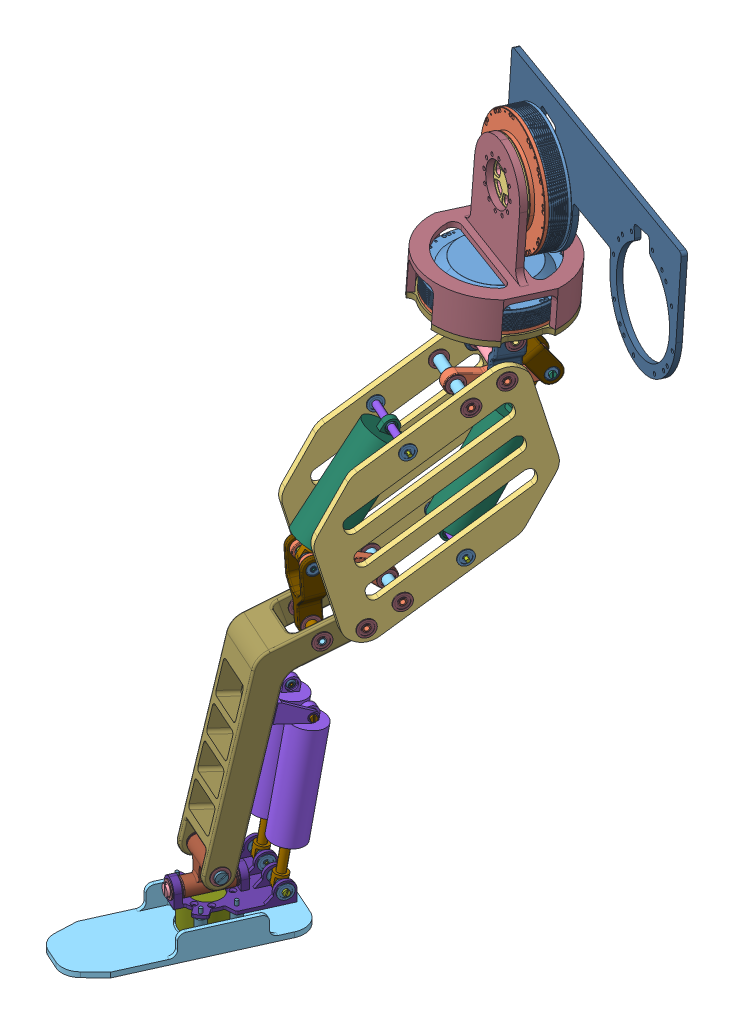
SolidWorks assembly 腿部总装, configuration 默认. Lengths in mm. (continued)
Mates (geometry in assembly coordinates): (continued)
- 同心60: concentric anti-aligned: cylinder of 轴承_NSK635-11 through (543.2359 479.3983 -8003.7197) axis (-0.911939 0 -0.410325) radius 2.5; cylinder of 膝关节5mm轴套2-3 through (539.2336 479.3983 -8005.5205) axis (0.911939 0 0.410325) radius 5
- 重合124: coincident anti-aligned: plane of 轴承_NSK635-14 through (539.0094 476.9588 -8005.0222) normal (0.911939 0 0.410325); plane of 膝关节5mm轴套2-3 through (539.2336 479.3983 -8005.5205) normal (-0.911939 0 -0.410325)
- 同心61: concentric aligned: circle of 膝髋推杆-1/脚踝推杆球头-2; cylinder of 膝关节5mm轴套3-2 through (526.0105 479.3983 -8011.4702) axis (0.911939 0 0.410325) radius 5
- 重合125: coincident anti-aligned: plane of 膝髋推杆-1/脚踝推杆球头-2 through (526.0105 479.3983 -8011.4702) normal (0.911939 0 0.410325); plane of 膝关节5mm轴套3-2 through (526.0105 479.3983 -8011.4702) normal (-0.911939 0 -0.410325)
- 同心62: concentric aligned: cylinder of 大腿侧板-1 through (511.6182 660.5079 -8116.57) axis (-0.911939 0 -0.410325) radius 9.5; cylinder of 轴承_NSK635-16 through (509.3577 659.5509 -8117.9101) axis (-0.911939 0 -0.410325) radius 9.5
- 重合126: coincident aligned: plane of 大腿侧板-1 through (425.784 514.1163 -7935.5535) normal (-0.911939 0 -0.410325); plane of 轴承_NSK635-16 through (507.193 650.3066 -8116.4834) normal (-0.911939 0 -0.410325)
- 同心63: concentric anti-aligned: cylinder of 大腿侧板-1 through (511.6182 660.5079 -8116.57) axis (0.911939 0 0.410325) radius 9.5; cylinder of 轴承_NSK635-15 through (513.0055 659.5509 -8116.2688) axis (-0.911939 0 -0.410325) radius 9.5
- 重合127: coincident aligned: plane of 大腿侧板-1 through (434.9033 514.1163 -7931.4502) normal (0.911939 0 0.410325); plane of 轴承_NSK635-15 through (516.5522 651.7135 -8112.9131) normal (0.911939 0 0.410325)
- 同心64: concentric anti-aligned: cylinder of 轴承_NSK635-15 through (513.0055 659.5509 -8116.2688) axis (-0.911939 0 -0.410325) radius 2.5; cylinder of 膝关节5mm轴套4-1 through (518.4578 660.5079 -8113.4926) axis (0.911939 0 0.410325) radius 5
- 重合128: coincident anti-aligned: plane of 膝髋推杆-1/脚踝推杆球头-1 through (559.5325 633.0528 -8107.9058) normal (-0.911939 0 -0.410325); plane of 膝关节5mm轴套4-1 through (559.5325 633.0528 -8107.9058) normal (0.911939 0 0.410325)
- 同心65: concentric anti-aligned: cylinder of 大腿侧板-1 through (543.7977 674.861 -8197.8367) axis (0.911939 0 0.410325) radius 11; cylinder of 膝关节U型架后侧-2 through (629.6228 674.861 -8159.2199) axis (-0.911939 0 -0.410325) radius 11
- 重合129: coincident aligned: plane of 膝关节U型架后侧-1 through (553.0875 467.2754 -8064.9462) normal (0.911939 0 0.410325); plane of 膝关节U型架后侧-2 through (621.3197 658.4644 -8216.5909) normal (0.911939 0 0.410325)
- 同心66: concentric aligned: cylinder of 膝髋推杆-2/脚踝推杆球头-2 through (633.731 675.7893 -8275.2477) axis (0.911939 0 0.410325) radius 2.5; cylinder of 膝关节U型架后侧-2 through (650.6019 675.7893 -8267.6567) axis (0.911939 0 0.410325) radius 9.5
- 同心67: concentric anti-aligned: cylinder of 膝关节U型架后侧-2 through (650.6019 675.7893 -8267.6567) axis (0.911939 0 0.410325) radius 9.5; cylinder of 轴承_NSK635-19 through (651.8683 675.7893 -8267.0868) axis (-0.911939 0 -0.410325) radius 9.5
- 重合130: coincident aligned: plane of 膝关节U型架后侧-2 through (656.536 664.3447 -8266.2225) normal (0.911939 0 0.410325); plane of 轴承_NSK635-19 through (655.356 667.9828 -8263.6001) normal (0.911939 0 0.410325)
- 同心68: concentric aligned: cylinder of 膝关节U型架后侧-2 through (626.8915 675.7893 -8278.3251) axis (-0.911939 0 -0.410325) radius 9.5; cylinder of 轴承_NSK635-20 through (622.6862 675.7893 -8280.2172) axis (-0.911939 0 -0.410325) radius 9.5
- 重合131: coincident aligned: plane of 膝关节U型架后侧-2 through (602.1794 659.6159 -8238.0256) normal (-0.911939 0 -0.410325); plane of 轴承_NSK635-20 through (620.5678 666.519 -8278.8934) normal (-0.911939 0 -0.410325)
- 距离5: distance = 6.5 mm anti-aligned: plane of 膝髋推杆-2/脚踝推杆球头-2 through (634.6429 675.7893 -8274.8373) normal (-0.911939 0 -0.410325); plane of 膝关节U型架后侧-2 through (629.1778 664.3447 -8278.5323) normal (0.911939 0 0.410325)
- 重合133: coincident aligned: circle of 膝关节U型架后侧-2; circle of 轴承_NSK6900NR-27
- 重合134: coincident aligned: circle of 膝关节U型架后侧-2; circle of 轴承_NSK6900NR-26
- 同心69: concentric aligned: cylinder of 大腿侧板-1 through (544.8687 471.6931 -8190.4684) axis (0.911939 0 0.410325) radius 9.5; cylinder of 膝髋推杆-2/脚踝推杆球头-1 through (587.0459 471.6931 -8171.4909) axis (0.911939 0 0.410325) radius 2.5
- 同心70: concentric anti-aligned: cylinder of 大腿侧板-1 through (524.9446 487.9356 -8146.1876) axis (0.911939 0 0.410325) radius 9.5; cylinder of 轴承_NSK635-22 through (526.8516 487.2218 -8147.0414) axis (-0.911939 0 -0.410325) radius 9.5
- 重合135: coincident aligned: plane of 大腿侧板-1 through (434.9033 514.1163 -7931.4502) normal (0.911939 0 0.410325); plane of 轴承_NSK635-22 through (530.5858 479.3045 -8144.1025) normal (0.911939 0 0.410325)
- 同心71: concentric aligned: cylinder of 大腿侧板-1 through (524.9446 487.9356 -8146.1876) axis (-0.911939 0 -0.410325) radius 9.5; cylinder of 轴承_NSK635-23 through (523.2038 487.2218 -8148.6827) axis (-0.911939 0 -0.410325) radius 9.5
- 重合136: coincident aligned: plane of 大腿侧板-1 through (425.784 514.1163 -7935.5535) normal (-0.911939 0 -0.410325); plane of 轴承_NSK635-23 through (521.3781 477.82 -8148.0095) normal (-0.911939 0 -0.410325)
- 重合137: coincident anti-aligned: plane of 膝髋推杆-2/脚踝推杆球头-1 through (587.9578 471.6931 -8171.0806) normal (-0.911939 0 -0.410325); plane of 膝关节5mm轴套4-3 through (587.9578 471.6931 -8171.0806) normal (0.911939 0 0.410325)
- 同心72: concentric aligned: cylinder of 膝髋推杆-2/脚踝推杆球头-1 through (587.0459 471.6931 -8171.4909) axis (0.911939 0 0.410325) radius 2.5; cylinder of 膝关节5mm轴套4-3 through (551.7082 471.6931 -8187.391) axis (0.911939 0 0.410325) radius 5
- 重合138: coincident anti-aligned: plane of 轴承_NSK635-22 through (530.9096 484.7476 -8144.8222) normal (0.911939 0 0.410325); plane of 膝关节5mm轴套4-3 through (531.7841 487.9356 -8143.1102) normal (-0.911939 0 -0.410325)
- 同心74: concentric anti-aligned: cylinder of 法兰轴承10_22_6-17 through (492.4155 404.6089 -8083.912) axis (-0.911939 0 -0.410325) radius 5; cylinder of 膝关节10mm轴套-1 through (515.7714 404.6089 -8073.403) axis (0.911939 0 0.410325) radius 7.5
- 同心75: concentric anti-aligned: cylinder of 大腿侧板-1 through (561.4995 700.1369 -8237.1785) axis (0.911939 0 0.410325) radius 11; cylinder of 法兰轴承10_22_6-29 through (561.398 700.1369 -8237.2241) axis (-0.911939 0 -0.410325) radius 11
- 重合139: coincident anti-aligned: plane of 大腿侧板-1 through (445.6606 446.5602 -7979.729) normal (-0.911939 0 -0.410325); plane of 法兰轴承10_22_6-29 through (561.4995 700.1369 -8237.1785) normal (0.911939 0 0.410325)
- 同心76: concentric anti-aligned: cylinder of 大腿侧板-1 through (543.7977 674.861 -8197.8367) axis (0.911939 0 0.410325) radius 11; cylinder of 法兰轴承10_22_6-28 through (543.6962 674.861 -8197.8824) axis (-0.911939 0 -0.410325) radius 11
- 重合140: coincident anti-aligned: plane of 大腿侧板-1 through (445.6606 446.5602 -7979.729) normal (-0.911939 0 -0.410325); plane of 法兰轴承10_22_6-28 through (543.7977 674.861 -8197.8367) normal (0.911939 0 0.410325)
- 同心77: concentric aligned: cylinder of 大腿侧板-1 through (543.7977 674.861 -8197.8367) axis (0.911939 0 0.410325) radius 11; cylinder of 法兰轴承10_22_6-31 through (553.0186 674.861 -8193.6878) axis (0.911939 0 0.410325) radius 11
- 重合141: coincident anti-aligned: plane of 大腿侧板-1 through (454.78 446.5602 -7975.6258) normal (0.911939 0 0.410325); plane of 法兰轴承10_22_6-31 through (552.9171 674.861 -8193.7334) normal (-0.911939 0 -0.410325)
- 同心78: concentric aligned: cylinder of 大腿侧板-1 through (561.4995 700.1369 -8237.1785) axis (0.911939 0 0.410325) radius 11; cylinder of 法兰轴承10_22_6-30 through (570.7204 700.1369 -8233.0295) axis (0.911939 0 0.410325) radius 11
- 重合142: coincident anti-aligned: plane of 大腿侧板-1 through (454.78 446.5602 -7975.6258) normal (0.911939 0 0.410325); plane of 法兰轴承10_22_6-30 through (570.6189 700.1369 -8233.0752) normal (-0.911939 0 -0.410325)
- 同心79: concentric aligned: cylinder of 法兰轴承10_22_6-31 through (553.0186 674.861 -8193.6878) axis (0.911939 0 0.410325) radius 5; cylinder of 膝关节10mm轴套2-3 through (554.285 674.861 -8193.118) axis (0.911939 0 0.410325) radius 7.5
- 重合143: coincident anti-aligned: plane of 法兰轴承10_22_6-31 through (558.4754 678.9486 -8202.431) normal (0.911939 0 0.410325); plane of 膝关节10mm轴套2-3 through (554.285 674.861 -8193.118) normal (-0.911939 0 -0.410325)
- 同心80: concentric anti-aligned: cylinder of 轴承_NSK635-19 through (651.8683 675.7893 -8267.0868) axis (-0.911939 0 -0.410325) radius 2.5; cylinder of 膝关节U型架-2 through (658.8093 675.7893 -8263.9637) axis (0.911939 0 0.410325) radius 9.5
- 同心82: concentric anti-aligned: cylinder of 小腿骨-1 through (477.5174 389.5165 -8038.3445) axis (0.911939 0 0.410325) radius 11; cylinder of 法兰轴承10_22_6-33 through (485.6234 389.5165 -8034.6973) axis (-0.911939 0 -0.410325) radius 11
- 重合145: coincident anti-aligned: plane of 小腿骨-1 through (427.5818 102.7196 -7905.4298) normal (-0.911939 0 -0.410325); plane of 法兰轴承10_22_6-33 through (485.7249 389.5165 -8034.6516) normal (0.911939 0 0.410325)
- 同心83: concentric aligned: cylinder of 小腿骨-1 through (477.5174 389.5165 -8038.3445) axis (0.911939 0 0.410325) radius 11; cylinder of 法兰轴承10_22_6-32 through (494.9457 389.5165 -8030.5027) axis (0.911939 0 0.410325) radius 11
- 重合146: coincident anti-aligned: plane of 小腿骨-1 through (527.9345 368.3725 -8104.0907) normal (0.911939 0 0.410325); plane of 法兰轴承10_22_6-32 through (494.8442 389.5165 -8030.5484) normal (-0.911939 0 -0.410325)
- 同心84: concentric aligned: cylinder of 膝关节U型架-1 through (535.4255 389.5165 -8012.2889) axis (-0.911939 0 -0.410325) radius 11; cylinder of 法兰轴承10_22_6-34 through (517.0853 389.5165 -8020.5411) axis (-0.911939 0 -0.410325) radius 11
- 重合148: coincident anti-aligned: plane of 膝关节U型架-1 through (523.3336 390.2848 -8034.1565) normal (-0.911939 0 -0.410325); plane of 法兰轴承10_22_6-34 through (517.1868 389.5165 -8020.4954) normal (0.911939 0 0.410325)
- 同心85: concentric aligned: cylinder of 小腿骨-1 through (477.5174 389.5165 -8038.3445) axis (0.911939 0 0.410325) radius 11; cylinder of 法兰轴承10_22_6-37 through (530.5114 389.5165 -8014.5) axis (0.911939 0 0.410325) radius 5
- 重合149: coincident anti-aligned: plane of 小腿骨-1 through (507.2619 141.7818 -7879.0201) normal (0.911939 0 0.410325); plane of 法兰轴承10_22_6-36 through (561.8718 389.5165 -8000.3895) normal (-0.911939 0 -0.410325)
- 同心86: concentric aligned: cylinder of 法兰轴承10_22_6-32 through (494.9457 389.5165 -8030.5027) axis (0.911939 0 0.410325) radius 5; cylinder of 膝关节10mm轴套3-1 through (496.2122 389.5165 -8029.9329) axis (0.911939 0 0.410325) radius 5.1
- 重合150: coincident anti-aligned: plane of 法兰轴承10_22_6-34 through (513.34 387.118 -8015.6016) normal (-0.911939 0 -0.410325); plane of 膝关节10mm轴套3-1 through (515.8188 389.5165 -8021.1109) normal (0.911939 0 0.410325)
- 同心87: concentric anti-aligned: cylinder of 膝关节U型架-2 through (628.7554 748.7562 -8219.7126) axis (-0.911939 0 -0.410325) radius 11; cylinder of 法兰轴承10_22_6-39 through (623.8413 748.7562 -8221.9238) axis (0.911939 0 0.410325) radius 11
- 重合151: coincident anti-aligned: plane of 膝关节U型架-2 through (625.9559 715.6529 -8226.8947) normal (0.911939 0 0.410325); plane of 法兰轴承10_22_6-39 through (623.7398 748.7562 -8221.9694) normal (-0.911939 0 -0.410325)
- 同心88: concentric aligned: cylinder of 膝关节U型架-2 through (628.7554 748.7562 -8219.7126) axis (-0.911939 0 -0.410325) radius 11; cylinder of 法兰轴承10_22_6-38 through (610.4151 748.7562 -8227.9648) axis (-0.911939 0 -0.410325) radius 11
- 重合152: coincident anti-aligned: plane of 膝关节U型架-2 through (605.5266 739.9752 -8216.8289) normal (-0.911939 0 -0.410325); plane of 法兰轴承10_22_6-38 through (610.5166 748.7562 -8227.9191) normal (0.911939 0 0.410325)
- 同心89: concentric aligned: cylinder of 法兰轴承10_22_6-30 through (570.7204 700.1369 -8233.0295) axis (0.911939 0 0.410325) radius 5; cylinder of 膝关节10mm轴套-2 through (-431.1082 141.1617 870.583) axis (0.002571 -0.999927 -0.011812) radius 7.5
- 同心90: concentric anti-aligned: circle of 膝髋推杆-2/脚踝推杆球头-2; line of 膝关节5mm轴套3-4 through (626.8915 675.7893 -8278.3251) axis (0.911939 0 0.410325)
- 重合154: coincident anti-aligned: plane of 轴承_NSK635-20 through (626.6672 673.3498 -8277.8268) normal (0.911939 0 0.410325); plane of 膝关节5mm轴套3-4 through (626.8915 675.7893 -8278.3251) normal (-0.911939 0 -0.410325)
- 同心91: concentric anti-aligned: cylinder of 膝关节U型架-2 through (618.684 675.7893 -8282.018) axis (-0.911939 0 -0.410325) radius 9.5; cylinder of 轴承_NSK635-28 through (617.4176 675.7893 -8282.5879) axis (0.911939 0 0.410325) radius 9.5
- 重合155: coincident aligned: plane of 膝关节U型架-2 through (598.7943 698.83 -8252.4361) normal (-0.911939 0 -0.410325); plane of 轴承_NSK635-28 through (612.4559 668.0046 -8282.7987) normal (-0.911939 0 -0.410325)
- 重合156: coincident anti-aligned: plane of 轴承_NSK635-20 through (621.0611 671.886 -8279.9897) normal (-0.911939 0 -0.410325); plane of 膝关节5mm轴套2-5 through (621.4198 675.7893 -8280.7871) normal (0.911939 0 0.410325)
- 同心93: concentric aligned: cylinder of 膝关节5mm轴套2-5 through (618.684 675.7893 -8282.018) axis (0.911939 0 0.410325) radius 5; cylinder of 轴承_NSK635-28 through (617.4176 675.7893 -8282.5879) axis (0.911939 0 0.410325) radius 2.5
- 同心94: concentric aligned: cylinder of 法兰轴承10_22_6-39 through (623.8413 748.7562 -8221.9238) axis (0.911939 0 0.410325) radius 5; cylinder of 髋关节座-1 through (523.6078 748.7562 -8267.0236) axis (0.911939 0 0.410325) radius 11
- 同心95: concentric aligned: line of 法兰轴承10_22_6-30 through (566.5152 700.1369 -8234.9217) axis (0.911939 0 0.410325); cylinder of 髋关节座-1 through (518.8197 700.1369 -8256.3821) axis (0.911939 0 0.410325) radius 11
- 同心96: concentric anti-aligned: cylinder of 髋关节座-1 through (523.6078 748.7562 -8267.0236) axis (0.911939 0 0.410325) radius 11; cylinder of 法兰轴承10_22_6-44 through (569.8338 748.7562 -8246.2243) axis (-0.911939 0 -0.410325) radius 11
- 重合158: coincident aligned: plane of 髋关节座-1 through (554.5139 685.9312 -8211.9047) normal (-0.911939 0 -0.410325); circle of 轴承_NSK6900NR-44
- 同心98: concentric anti-aligned: cylinder of 髋关节座-1 through (518.8197 700.1369 -8256.3821) axis (0.911939 0 0.410325) radius 11; cylinder of 法兰轴承10_22_6-45 through (574.4729 700.092 -8232.1478) axis (-0.904587 -0.001074 -0.426287) radius 11
- 重合159: coincident anti-aligned: plane of 髋关节座-1 through (614.8284 678.3084 -8321.5817) normal (-0.911939 0 -0.410325); plane of 法兰轴承10_22_6-45 through (574.5736 700.0921 -8232.1003) normal (0.904587 0.001074 0.426287)
- 同心99: concentric aligned: cylinder of 髋关节座-1 through (523.6078 748.7562 -8267.0236) axis (0.911939 0 0.410325) radius 11; cylinder of 法兰轴承10_22_6-46 through (580.0682 748.7562 -8241.6194) axis (0.911939 0 0.410325) radius 11
- 重合160: coincident anti-aligned: plane of 髋关节座-1 through (622.5939 757.4371 -8336.4032) normal (0.911939 0 0.410325); plane of 法兰轴承10_22_6-46 through (579.9667 748.7562 -8241.665) normal (-0.911939 0 -0.410325)
- 同心100: concentric aligned: cylinder of 髋关节座-1 through (518.8197 700.1369 -8256.3821) axis (0.911939 0 0.410325) radius 11; cylinder of 法兰轴承10_22_6-47 through (584.3995 700.1369 -8226.8747) axis (0.911939 0 0.410325) radius 11
- 重合161: coincident anti-aligned: plane of 髋关节座-1 through (610.9347 680.3818 -8286.1199) normal (0.911939 0 0.410325); plane of 法兰轴承10_22_6-47 through (584.298 700.1369 -8226.9203) normal (-0.911939 0 -0.410325)
- 同心101: concentric aligned: cylinder of 法兰轴承10_22_6-47 through (584.3995 700.1369 -8226.8747) axis (0.911939 0 0.410325) radius 5; cylinder of 膝关节10mm轴套-3 through (585.6659 700.1369 -8226.3048) axis (0.911939 0 0.410325) radius 7.5
- 重合162: coincident anti-aligned: plane of 法兰轴承10_22_6-48 through (641.5441 702.1955 -8207.9233) normal (-0.911939 0 -0.410325); plane of 膝关节10mm轴套-3 through (639.0143 700.1369 -8202.3008) normal (0.911939 0 0.410325)
- 同心103: concentric aligned: cylinder of 法兰轴承10_22_6-46 through (580.0682 748.7562 -8241.6194) axis (0.911939 0 0.410325) radius 5; cylinder of 髋关节10mm轴套-1 through (581.3346 748.7562 -8241.0496) axis (0.911939 0 0.410325) radius 7.5
- 重合164: coincident anti-aligned: plane of 法兰轴承10_22_6-38 through (611.5154 758.1228 -8233.7945) normal (-0.911939 0 -0.410325); plane of 髋关节10mm轴套-1 through (609.1487 748.7562 -8228.5346) normal (0.911939 0 0.410325)
- 重合166: coincident anti-aligned: plane of 法兰轴承10_22_6-46 through (578.8584 746.341 -8235.5464) normal (0.911939 0 0.410325); plane of 髋关节10mm轴套-1 through (581.3346 748.7562 -8241.0496) normal (-0.911939 0 -0.410325)
- 重合168: coincident anti-aligned: plane of 膝关节5mm轴套2-5 through (618.684 675.7893 -8282.018) normal (-0.911939 0 -0.410325); plane of 轴承_NSK635-28 through (618.3058 671.897 -8281.1774) normal (0.911939 0 0.410325)
- 重合169: coincident anti-aligned: plane of B1电机模型-220923.STEP-1/B1________-220923.STEP.STEP-1/11UXMR1_DVUR40_RDCR1_HLDR1_BHDR1.STEP.STEP-1 through (654.6158 772.5963 -8229.7314) normal (-0.025023 -0.998139 0.055612); plane of 髋关节座-1 through (614.1978 774.2391 -8218.4315) normal (0.025023 0.998139 -0.055612)
- 同心104: concentric anti-aligned: cylinder of B1电机模型-220923.STEP-1/B1________-220923.STEP.STEP-1/11UXMR1_DVUR40_HOSR1_BASR1.STEP.STEP-1 through (613.3795 741.6 -8216.613) axis (-0.025023 -0.998139 0.055612) radius 85.25; cylinder of 髋关节座-1 through (611.9458 684.4067 -8213.4264) axis (0.025023 0.998139 -0.055612) radius 30
- 重合170: coincident anti-aligned: plane of B1电机模型-220923.STEP-1/B1________-220923.STEP.STEP-1/11UXMR1_DVUR40_HOSR1_BASR1.STEP.STEP-1 through (559.2029 783.9744 -8239.2727) normal (-0.025023 -0.998139 0.055612); plane of 髋关节电机固定座-1 through (614.4355 783.7215 -8218.9598) normal (0.025023 0.998139 -0.055612)
- 同心105: concentric aligned: cylinder of B1电机模型-220923.STEP-1/B1________-220923.STEP.STEP-1/11UXMR1_DVUR40_HOSR1_BASR1.STEP.STEP-1 through (613.3795 741.6 -8216.613) axis (-0.025023 -0.998139 0.055612) radius 85.25; cylinder of 髋关节电机固定座-1 through (614.4355 783.7215 -8218.9598) axis (-0.025023 -0.998139 0.055612) radius 87.5
- 同心106: concentric aligned: cylinder of 髋关节电机固定座-1 through (612.0457 688.3939 -8213.6486) axis (0.025023 0.998139 -0.055612) radius 98; cylinder of 髋关节电机固定座2-1 through (614.4355 783.7215 -8218.9598) axis (0.025023 0.998139 -0.055612) radius 98
- 重合171: coincident anti-aligned: plane of 髋关节电机固定座-1 through (614.4355 783.7215 -8218.9598) normal (0.025023 0.998139 -0.055612); plane of 髋关节电机固定座2-1 through (614.4355 783.7215 -8218.9598) normal (-0.025023 -0.998139 0.055612)
- 同心107: concentric anti-aligned: cylinder of 髋关节电机固定座-1 through (604.1766 683.4356 -8306.1823) axis (0.025023 0.998139 -0.055612) radius 2.75; cylinder of 髋关节电机固定座2-1 through (606.5664 778.7631 -8311.4936) axis (-0.025023 -0.998139 0.055612) radius 2.1
- 同心108: concentric aligned: cylinder of B1电机模型-220923-1/B1电机模型-220923.STEP-1/B1________-220923.STEP.STEP-1/11UXMR1_DVUR40_HOSR1_BASR1.STEP.STEP-1 through (608.38 931.1652 -8200.6588) axis (-0.344283 0.060831 0.936893) radius 58.85; cylinder of 髋关节电机固定座2-1 through (680.7483 918.3785 -8397.5938) axis (-0.344283 0.060831 0.936893) radius 30
- 同心109: concentric aligned: cylinder of B1电机模型-220923-1/B1电机模型-220923.STEP-1/B1________-220923.STEP.STEP-1/11UXMR1_DVUR40_RDCR1_HLDR1_BHDR1.STEP.STEP-1 through (592.2673 911.5712 -8244.9066) axis (-0.344283 0.060831 0.936893) radius 3.75; cylinder of 髋关节电机固定座2-1 through (651.8627 901.0414 -8407.0828) axis (-0.344283 0.060831 0.936893) radius 2.75
- 同心110: concentric anti-aligned: cylinder of B1电机模型-220923.STEP-1/B1________-220923.STEP.STEP-1/11UXMR1_DVUR40_HOSR1_BASR1.STEP.STEP-1 through (614.1423 788.2487 -8137.8366) axis (-0.025023 -0.998139 0.055612) radius 2.5; cylinder of 髋关节电机固定座-1 through (613.8921 778.2673 -8137.2805) axis (0.025023 0.998139 -0.055612) radius 2.75
- 同心111: concentric aligned: cylinder of 脚掌-1 through (499.0075 0 -7871.6683) axis (0 1 0) radius 2.05; cylinder of 六轴力_力矩传感器安装板-1 through (499.0075 47 -7871.6683) axis (0 1 0) radius 2.6
- 同心112: concentric anti-aligned: cylinder of 橡胶减震套-4 through (499.0075 58 -7871.6683) axis (0 -1 0) radius 2.5; cylinder of 六轴力_力矩传感器安装板-1 through (499.0075 47 -7871.6683) axis (0 1 0) radius 2.6
- 同心113: concentric anti-aligned: cylinder of 六轴力_力矩传感器安装板-1 through (447.5083 64 -7847.9675) axis (0.410325 0 -0.911939) radius 11; cylinder of 法兰轴承10_22_6-52 through (455.3594 64 -7865.4164) axis (-0.410325 0 0.911939) radius 11
- 重合173: coincident anti-aligned: plane of 六轴力_力矩传感器安装板-1 through (441.726 8.0178 -7871.6728) normal (-0.410325 0 0.911939); plane of 法兰轴承10_22_6-52 through (455.4051 64 -7865.5179) normal (0.410325 0 -0.911939)
- 同心114: concentric aligned: cylinder of 六轴力_力矩传感器安装板-1 through (447.5083 64 -7847.9675) axis (0.410325 0 -0.911939) radius 11; cylinder of 法兰轴承10_22_6-53 through (459.554 64 -7874.7388) axis (0.410325 0 -0.911939) radius 11
- 重合174: coincident anti-aligned: plane of 六轴力_力矩传感器安装板-1 through (473.1874 81 -7868.4824) normal (0.410325 0 -0.911939); plane of 法兰轴承10_22_6-53 through (459.5083 64 -7874.6373) normal (-0.410325 0 0.911939)
- 同心116: concentric anti-aligned: cylinder of 脚踝交叉转轴套筒-1 through (486.5898 64 -7934.8253) axis (-0.410325 0 0.911939) radius 13; cylinder of 法兰轴承10_22_6-53 through (459.554 64 -7874.7388) axis (0.410325 0 -0.911939) radius 5
- 重合175: coincident anti-aligned: plane of 六轴力_力矩传感器安装板-1 through (474.552 81 -7944.6279) normal (-0.410325 0 0.911939); plane of 法兰轴承10_22_6-54 through (488.2311 64 -7938.4731) normal (0.410325 0 -0.911939)
- 同心117: concentric anti-aligned: cylinder of 六轴力_力矩传感器安装板-1 through (447.5083 64 -7847.9675) axis (0.410325 0 -0.911939) radius 11; cylinder of 法兰轴承10_22_6-54 through (488.1854 64 -7938.3716) axis (-0.410325 0 0.911939) radius 11
- 同心118: concentric aligned: cylinder of 六轴力_力矩传感器安装板-1 through (447.5083 64 -7847.9675) axis (0.410325 0 -0.911939) radius 11; cylinder of 法兰轴承10_22_6-55 through (492.38 64 -7947.6939) axis (0.410325 0 -0.911939) radius 11
- 重合176: coincident anti-aligned: plane of 六轴力_力矩传感器安装板-1 through (478.6552 8.0178 -7953.7473) normal (0.410325 0 -0.911939); plane of 法兰轴承10_22_6-55 through (492.3343 64 -7947.5924) normal (-0.410325 0 0.911939)
- 重合177: coincident anti-aligned: plane of B1电机模型-220923-1/B1电机模型-220923.STEP-1/B1________-220923.STEP.STEP-1/11UXMR1_DVUR40_RDCR1_HLDR1_BHDR1.STEP.STEP-1 through (582.5095 889.16 -8242.8745) normal (-0.344283 0.060831 0.936893); plane of 髋关节电机固定座2-1 through (564.9996 989.2917 -8255.8103) normal (0.344283 -0.060831 -0.936893)
- 距离6: distance = 38 mm anti-aligned: plane of 六轴力_力矩传感器安装板-1 through (473.8697 46 -7906.5552) normal (0 -1 0); plane of 脚掌-1 through (445.8363 8 -7716.3043) normal (0 1 0)
- 重合184: coincident anti-aligned: plane of 踝关节5mm轴套-4 through (481.3896 64 -7985.4139) normal (-0.911939 0 -0.410325); plane of 脚踝推杆-4/脚踝推杆球头-1 through (481.3896 64 -7985.4139) normal (0.911939 0 0.410325)
- 重合185: coincident anti-aligned: plane of 小腿骨-1 through (507.2619 141.7818 -7879.0201) normal (0.911939 0 0.410325); plane of 法兰轴承10_22_6-13 through (581.4311 404.6089 -8043.8596) normal (-0.911939 0 -0.410325)
- 重合187: coincident anti-aligned: plane of 脚掌-1 through (445.8363 0 -7716.3043) normal (0 -1 0)
- 同心123: concentric anti-aligned: cylinder of 六轴力_力矩传感器安装板-1 through (516.6515 47 -7910.8817) axis (0 1 0) radius 2.6; cylinder of 橡胶减震套-1 through (516.6515 58 -7910.8817) axis (0 -1 0) radius 2.5
- 重合188: coincident anti-aligned: plane of 六轴力_力矩传感器安装板-1 through (473.8697 46 -7906.5552) normal (0 -1 0); plane of 橡胶减震套-1 through (516.6515 46 -7910.8817) normal (0 1 0)
- 同心124: concentric anti-aligned: cylinder of 六轴力_力矩传感器安装板-1 through (448.7319 47 -7941.442) axis (0 1 0) radius 2.6; cylinder of 橡胶减震套-2 through (448.7319 58 -7941.442) axis (0 -1 0) radius 2.5
- 重合189: coincident anti-aligned: plane of 六轴力_力矩传感器安装板-1 through (473.8697 46 -7906.5552) normal (0 -1 0); plane of 橡胶减震套-2 through (448.7319 46 -7941.442) normal (0 1 0)
- 同心125: concentric anti-aligned: cylinder of 轴承_NSK635-2 through (580.6415 64 -8027.1442) axis (-0.911939 0 -0.410325) radius 9.5; cylinder of 六轴力_力矩传感器安装板-1 through (501.451 64 -8095.8014) axis (0.911939 0 0.410325) radius 9.5
- 重合190: coincident aligned: plane of 轴承_NSK635-2 through (585.2038 56.0475 -8026.0456) normal (0.911939 0 0.410325); plane of 六轴力_力矩传感器安装板-1 through (571.202 -122.6779 -8002.2382) normal (0.911939 0 0.410325)
- 同心127: concentric anti-aligned: cylinder of 轴承_NSK635-3 through (528.8639 64 -8050.4414) axis (0.911939 0 0.410325) radius 9.5; cylinder of 脚踝推杆-1/脚踝推杆伸缩杆-1 through (581.2455 63.9999 -8059.8976) axis (-0.911913 0.000017 -0.410383) radius 8
- 重合192: coincident anti-aligned: plane of 轴承_NSK635-2 through (579.5536 60.0237 -8028.1107) normal (-0.911939 0 -0.410325); plane of 踝关节5mm轴套-1 through (590.3651 64 -8055.7946) normal (0.911939 0 0.410325)
- 重合193: coincident anti-aligned: plane of 轴承_NSK635-2 through (584.9583 61.5148 -8025.5) normal (0.911939 0 0.410325); plane of 脚踝推杆轴-1 through (595.8367 64 -8053.3327) normal (-0.911939 0 -0.410325)
- 重合194: coincident anti-aligned: plane of 轴承_NSK635-1 through (549.3289 61.5027 -8041.3611) normal (0.911939 0 0.410325); plane of 踝关节5mm轴套-2 through (563.0069 64 -8068.1044) normal (-0.911939 0 -0.410325)
- 同心128: concentric anti-aligned: cylinder of 六轴力_力矩传感器安装板-1 through (499.0075 47 -7871.6683) axis (0 1 0) radius 2.6; cylinder of 橡胶减震套-4 through (499.0075 58 -7871.6683) axis (0 -1 0) radius 2.5
- 重合195: coincident anti-aligned: plane of 六轴力_力矩传感器安装板-1 through (473.8697 46 -7906.5552) normal (0 -1 0); plane of 橡胶减震套-4 through (499.0075 46 -7871.6683) normal (0 1 0)
- 同心129: concentric anti-aligned: cylinder of 六轴力_力矩传感器安装板-1 through (431.0879 47 -7902.2286) axis (0 1 0) radius 2.6; cylinder of 橡胶减震套-3 through (431.0879 58 -7902.2286) axis (0 -1 0) radius 2.5
- 重合196: coincident anti-aligned: plane of 六轴力_力矩传感器安装板-1 through (473.8697 46 -7906.5552) normal (0 -1 0); plane of 橡胶减震套-3 through (431.0879 46 -7902.2286) normal (0 1 0)
- 同心130: concentric anti-aligned: cylinder of 橡胶减震套-1 through (516.6515 16 -7910.8817) axis (0 1 0) radius 7.5; cylinder of 脚掌5mm轴套-1 through (516.6515 16 -7910.8817) axis (0 -1 0) radius 7.5
- 重合198: coincident anti-aligned: plane of 橡胶减震套-1 through (516.6515 16 -7910.8817) normal (0 -1 0); plane of 脚掌5mm轴套-1 through (516.6515 16 -7910.8817) normal (0 1 0)
- 重合203: coincident anti-aligned: plane of 踝关节5mm轴套-2 through (527.8985 64 -7964.4873) normal (0.911939 0 0.410325); plane of 脚踝推杆-1/脚踝推杆球头-1 through (527.8985 64 -7964.4873) normal (-0.911939 0 -0.410325)
- 重合204: coincident anti-aligned: plane of 法兰轴承10_22_6-20 through (521.3861 436.17 -8120.0007) normal (0.911939 0 0.410325); plane of 膝关节10mm轴套2-1 through (520.706 429.8849 -8118.4893) normal (-0.911939 0 -0.410325)
- 同心131: concentric aligned: cylinder of 髋关节座-1 through (518.8197 700.1369 -8256.3821) axis (0.911939 0 0.410325) radius 11; cylinder of 法兰轴承10_22_6-56 through (650.5151 700.1369 -8197.1261) axis (0.911939 0 0.410325) radius 11
- 重合206: coincident anti-aligned: plane of 髋关节座-1 through (690.9754 678.3084 -8287.3195) normal (0.911939 0 0.410325); plane of 法兰轴承10_22_6-56 through (650.4136 700.1369 -8197.1718) normal (-0.911939 0 -0.410325)
- 同心132: concentric aligned: cylinder of 法兰轴承10_22_6-10 through (505.1826 404.6089 -8078.1674) axis (-0.911939 0 -0.410325) radius 5; cylinder of 膝关节10mm轴套4-1 through (503.9162 404.6089 -8078.7372) axis (-0.911939 0 -0.410325) radius 5.1
- 同心133: concentric anti-aligned: cylinder of 小腿骨-1 through (497.0767 404.6089 -8081.8147) axis (0.911939 0 0.410325) radius 11; cylinder of 法兰轴承10_22_6-10 through (505.1826 404.6089 -8078.1674) axis (-0.911939 0 -0.410325) radius 11
- 重合207: coincident anti-aligned: plane of 小腿骨-1 through (427.5818 102.7196 -7905.4298) normal (-0.911939 0 -0.410325); plane of 法兰轴承10_22_6-10 through (505.2841 404.6089 -8078.1217) normal (0.911939 0 0.410325)
- 重合208: coincident anti-aligned: plane of 法兰轴承10_22_6-10 through (502.9023 398.597 -8076.4837) normal (-0.911939 0 -0.410325); plane of 膝关节10mm轴套4-1 through (503.9162 404.6089 -8078.7372) normal (0.911939 0 0.410325)
- 重合209: coincident anti-aligned: plane of 法兰轴承10_22_6-18 through (505.5042 406.8742 -8084.7036) normal (0.911939 0 0.410325); plane of 膝关节10mm轴套4-1 through (503.0043 404.6089 -8079.1476) normal (-0.911939 0 -0.410325)
- 同心134: concentric aligned: cylinder of 法兰轴承10_22_6-57 through (574.1651 700.1369 -8231.4796) axis (-0.911939 0 -0.410325) radius 5; cylinder of 膝关节10mm轴套4-2 through (572.8987 700.1369 -8232.0494) axis (-0.911939 0 -0.410325) radius 7.5
- 重合210: coincident anti-aligned: plane of 法兰轴承10_22_6-57 through (574.2973 705.6716 -8235.1576) normal (-0.911939 0 -0.410325); plane of 膝关节10mm轴套4-2 through (572.8987 700.1369 -8232.0494) normal (0.911939 0 0.410325)
- 同心135: concentric anti-aligned: cylinder of 轴承_NSK635-2 through (580.6415 64 -8027.1442) axis (-0.911939 0 -0.410325) radius 2.5; cylinder of 踝关节5mm轴套-1 through (580.7897 64 -8060.1031) axis (0.911939 0 0.410325) radius 4
- 同心136: concentric anti-aligned: cylinder of 脚踝交叉转轴套筒-1 through (530.6379 98.3066 -7881.0124) axis (-0.911939 0 -0.410325) radius 11; cylinder of 法兰轴承10_22_6-58 through (499.2775 98.3066 -7895.123) axis (0.911939 0 0.410325) radius 11
- 重合211: coincident anti-aligned: plane of 脚踝交叉转轴套筒-1 through (499.176 98.3066 -7895.1687) normal (0.911939 0 0.410325); plane of 法兰轴承10_22_6-58 through (499.176 98.3066 -7895.1687) normal (-0.911939 0 -0.410325)
- 同心137: concentric aligned: cylinder of 直径10轴-1 through (513.3111 98.3066 -7888.8086) axis (-0.911939 0 -0.410325) radius 5; cylinder of 膝关节10mm轴套4-5 through (501.4558 98.3066 -7894.1428) axis (-0.911939 0 -0.410325) radius 5.1
- 重合212: coincident anti-aligned: plane of 法兰轴承10_22_6-8 through (501.1688 104.7689 -7893.5048) normal (-0.911939 0 -0.410325); plane of 膝关节10mm轴套4-5 through (501.4558 98.3066 -7894.1428) normal (0.911939 0 0.410325)
- 重合213: coincident anti-aligned: plane of 法兰轴承10_22_6-58 through (501.9665 92.8085 -7897.7149) normal (0.911939 0 0.410325); plane of 膝关节10mm轴套4-5 through (500.5439 98.3066 -7894.5532) normal (-0.911939 0 -0.410325)
- 重合214: coincident aligned: circle of 脚踝交叉转轴套筒-1; circle of 法兰轴承10_22_6-60
- 同心138: concentric anti-aligned: cylinder of 法兰轴承10_22_6-60 through (486.6354 64 -7934.9268) axis (0.410325 0 -0.911939) radius 5; cylinder of 膝关节10mm轴套4-7 through (487.6156 64 -7937.1051) axis (-0.410325 0 0.911939) radius 5.1
- 重合215: coincident anti-aligned: plane of 法兰轴承10_22_6-60 through (484.8769 69.9776 -7937.2408) normal (0.410325 0 -0.911939); plane of 膝关节10mm轴套4-7 through (487.2053 64 -7936.1932) normal (-0.410325 0 0.911939)
- 重合216: coincident anti-aligned: plane of 法兰轴承10_22_6-54 through (487.8234 70.496 -7937.0116) normal (-0.410325 0 0.911939); plane of 膝关节10mm轴套4-7 through (487.6156 64 -7937.1051) normal (0.410325 0 -0.911939)
- 重合217: coincident anti-aligned: circle of 脚踝交叉转轴套筒-1; circle of 法兰轴承10_22_6-61
- 重合218: coincident anti-aligned: plane of 法兰轴承10_22_6-61 through (460.7552 74.9973 -7876.8177) normal (-0.410325 0 0.911939); plane of 膝关节10mm轴套4-8 through (460.5341 64 -7876.9171) normal (0.410325 0 -0.911939)
- 同心142: concentric aligned: cylinder of 法兰轴承10_22_6-61 through (461.1496 64 -7878.2851) axis (-0.410325 0 0.911939) radius 12.5; cylinder of 膝关节10mm轴套4-8 through (460.5341 64 -7876.9171) axis (-0.410325 0 0.911939) radius 7.5
- 同心143: concentric anti-aligned: cylinder of 脚掌-1 through (473.8697 0 -7906.5552) axis (0 1 0) radius 37.5; cylinder of 六轴力_力矩传感器-1 through (473.8697 46 -7906.5552) axis (0 -1 0) radius 35
- 同心144: concentric anti-aligned: cylinder of 轴承5_12_4-1 through (479.2425 312.4093 -8021.7345) axis (-0.911939 0 -0.410325) radius 2.5; cylinder of 脚踝推杆-4/脚踝推杆球头-2 through (488.4044 317.8695 -8025.375) axis (0.911939 0 0.410325) radius 2.5
- 重合219: coincident anti-aligned: plane of 小腿骨-1 through (507.2619 141.7818 -7879.0201) normal (0.911939 0 0.410325); plane of 法兰轴承5_11_5-1 through (557.4518 287.8759 -7990.566) normal (-0.911939 0 -0.410325)
- 同心146: concentric anti-aligned: cylinder of 法兰轴承5_11_5-1 through (558.0092 287.8759 -7990.3152) axis (0.911939 0 0.410325) radius 2.5; cylinder of 膝关节5mm轴套5-1 through (553.804 287.8759 -7992.2073) axis (-0.911939 0 -0.410325) radius 2.6
- 重合220: coincident anti-aligned: plane of 法兰轴承5_11_5-1 through (552.621 284.4208 -7989.5781) normal (-0.911939 0 -0.410325); plane of 膝关节5mm轴套5-1 through (553.804 287.8759 -7992.2073) normal (0.911939 0 0.410325)
- 同心147: concentric aligned: cylinder of 脚踝推杆-1/脚踝推杆球头-2 through (541.7208 287.8759 -7997.6441) axis (0.911939 0 0.410325) radius 2.5; cylinder of 法兰轴承5_11_5-1 through (558.0092 287.8759 -7990.3152) axis (0.911939 0 0.410325) radius 2.5
- 平行19: parallel aligned: plane of 小腿骨-1 through (507.2619 141.7818 -7879.0201) normal (0.911939 0 0.410325); plane of 六轴力_力矩传感器安装板-1 through (526.5183 -122.6779 -7902.9295) normal (0.911939 0 0.410325)
- 重合224: coincident anti-aligned: plane of 脚踝推杆-1/脚踝推杆球头-2 through (550.8402 287.8759 -7993.5409) normal (0.911939 0 0.410325); plane of 膝关节5mm轴套5-1 through (550.8402 287.8759 -7993.5409) normal (-0.911939 0 -0.410325)
- 重合225: coincident anti-aligned: plane of 脚踝推杆-4/脚踝推杆球头-2 through (487.9164 287.8759 -8021.8533) normal (-0.911939 0 -0.410325); plane of 膝关节5mm轴套5-2 through (487.9164 287.8759 -8021.8533) normal (0.911939 0 0.410325)
- 同心148: concentric anti-aligned: cylinder of 脚踝推杆-4/脚踝推杆球头-2 through (487.0044 287.8759 -8022.2637) axis (0.911939 0 0.410325) radius 2.5; cylinder of 膝关节5mm轴套5-2 through (487.9164 287.8759 -8021.8533) axis (-0.911939 0 -0.410325) radius 2.6
- 重合226: coincident anti-aligned: plane of 轴承5_12_4-1 through (483.8592 310.1192 -8020.7568) normal (0.911939 0 0.410325); plane of 膝关节5mm轴套5-2 through (486.3525 317.8695 -8026.2983) normal (-0.911939 0 -0.410325)
- 同心149: concentric aligned: cylinder of 大腿侧板-2 through (617.5064 487.9356 -8104.5396) axis (0.911939 0 0.410325) radius 9.5; cylinder of 轴承_NSK635-30 through (623.6363 487.3143 -8103.2694) axis (0.911939 0 0.410325) radius 9.5
- 重合227: coincident anti-aligned: plane of 大腿侧板-2 through (527.4652 514.1163 -7889.8022) normal (0.911939 0 0.410325); plane of 轴承_NSK635-30 through (623.5349 487.3143 -8103.3151) normal (-0.911939 0 -0.410325)
- 重合228: coincident aligned: circle of 大腿侧板-2; circle of 轴承_NSK635-31
- 重合229: coincident aligned: circle of 大腿侧板-2; circle of 轴承_NSK635-32
- 重合230: coincident aligned: circle of 大腿侧板-2; circle of 轴承_NSK635-33
- 重合231: coincident aligned: circle of 大腿侧板-1; circle of 法兰轴承5-19-6-1
- 重合232: coincident aligned: circle of 大腿侧板-1; circle of 法兰轴承5-19-6-4
- 同心150: concentric anti-aligned: cylinder of 大腿侧板-1 through (516.4433 633.0528 -8127.2937) axis (0.911939 0 0.410325) radius 9.5; cylinder of 法兰轴承5-19-6-2 through (512.6941 633.0528 -8128.9807) axis (-0.911939 0 -0.410325) radius 9.5
- 重合233: coincident anti-aligned: plane of 大腿侧板-1 through (445.6606 446.5602 -7979.729) normal (-0.911939 0 -0.410325); plane of 法兰轴承5-19-6-2 through (512.7956 633.0528 -8128.935) normal (0.911939 0 0.410325)
- 同心151: concentric aligned: cylinder of 大腿侧板-1 through (516.4433 633.0528 -8127.2937) axis (0.911939 0 0.410325) radius 9.5; cylinder of 法兰轴承5-19-6-3 through (522.0165 633.0528 -8124.7861) axis (0.911939 0 0.410325) radius 9.5
- 重合234: coincident anti-aligned: plane of 大腿侧板-1 through (454.78 446.5602 -7975.6258) normal (0.911939 0 0.410325); plane of 法兰轴承5-19-6-3 through (521.915 633.0528 -8124.8318) normal (-0.911939 0 -0.410325)
- 重合235: coincident aligned: circle of 六轴力_力矩传感器安装板-1; circle of 法兰轴承5-19-6-9
- 重合236: coincident aligned: circle of 六轴力_力矩传感器安装板-1; circle of 法兰轴承5-19-6-10
- 重合237: coincident anti-aligned: plane of 脚踝推杆轴-1 through (551.153 64 -7954.024) normal (-0.911939 0 -0.410325); plane of 法兰轴承5-19-6-9 through (548.3705 57.3468 -7947.84) normal (0.911939 0 0.410325)
- 同心153: concentric aligned: cylinder of 脚踝推杆轴-1 through (513.3075 64 -7971.0525) axis (-0.911939 0 -0.410325) radius 1.25; cylinder of 法兰轴承5-19-6-10 through (514.1179 64 -7970.6879) axis (-0.911939 0 -0.410325) radius 2.5
- 同心154: concentric aligned: cylinder of 脚踝推杆-4/脚踝推杆球头-1 through (472.2702 64 -7989.5172) axis (0.911939 0 0.410325) radius 2.5; cylinder of 六轴力_力矩传感器安装板-1 through (456.7673 64 -7996.4927) axis (0.911939 0 0.410325) radius 9.5
- 同心155: concentric aligned: cylinder of 踝关节5mm轴套-1 through (536.106 64 -7960.7944) axis (0.911939 0 0.410325) radius 4; cone of 脚踝推杆-1/脚踝推杆球头-1 through (536.106 64 -7960.7944) axis (0.911939 0 0.410325)
- 同心156: concentric anti-aligned: cylinder of 踝关节5mm轴套-2 through (518.3232 64 -7968.7957) axis (0.911939 0 0.410325) radius 4; cylinder of 脚踝推杆轴-1 through (551.153 64 -7954.024) axis (-0.911939 0 -0.410325) radius 2.5
- 重合238: coincident anti-aligned: plane of 踝关节5mm轴套-1 through (545.6813 64 -7956.486) normal (0.911939 0 0.410325); plane of 法兰轴承5-19-6-9 through (544.9491 62.2491 -7954.8586) normal (-0.911939 0 -0.410325)
- 重合239: coincident aligned: circle of 法兰轴承10_22_6-17; circle of 直径10轴2-3
- 重合240: coincident aligned: circle of 法兰轴承10_22_6-19; circle of 直径10轴2-2
- 重合241: coincident aligned: circle of 法兰轴承10_22_6-28; circle of 直径10轴2-1
- 重合242: coincident aligned: circle of 法兰轴承10_22_6-29; circle of 直径10轴2-4
- 重合243: coincident aligned: circle of 法兰轴承10_22_6-44; circle of 直径10轴3-1
- 重合244: coincident aligned: circle of 法兰轴承10_22_6-52; circle of 直径10轴4-1
- 同心157: concentric aligned: cylinder of 膝关节5mm轴套5-2 through (487.9164 287.8759 -8021.8533) axis (-0.911939 0 -0.410325) radius 2.6; cylinder of 法兰轴承5_11_5-2 through (480.7474 287.8759 -8025.079) axis (-0.911939 0 -0.410325) radius 2.5
- 重合245: coincident anti-aligned: plane of 膝关节5mm轴套5-2 through (484.9526 287.8759 -8023.1869) normal (-0.911939 0 -0.410325); plane of 法兰轴承5_11_5-2 through (484.2954 285.9564 -8021.7262) normal (0.911939 0 0.410325)
- 重合246: coincident anti-aligned: plane of 膝关节5mm轴套4-3 through (551.7082 471.6931 -8187.391) normal (-0.911939 0 -0.410325); plane of 法兰轴承5-19-6-4 through (552.3817 468.0453 -8188.8878) normal (0.911939 0 0.410325)
- 同心158: concentric anti-aligned: cylinder of 膝髋推杆-1/脚踝推杆球头-1 through (558.6205 633.0528 -8108.3162) axis (0.911939 0 0.410325) radius 2.5; cylinder of 法兰轴承5-19-6-2 through (512.6941 633.0528 -8128.9807) axis (-0.911939 0 -0.410325) radius 2.5
- 同心159: concentric aligned: cylinder of 膝髋推杆-1/脚踝推杆球头-1 through (558.6205 633.0528 -8108.3162) axis (0.911939 0 0.410325) radius 2.5; cylinder of 膝关节5mm轴套4-1 through (523.2829 633.0528 -8124.2163) axis (0.911939 0 0.410325) radius 5
- 重合248: coincident aligned: circle of 法兰轴承10_22_6-33; circle of 直径10轴5-1
- 同心160: concentric anti-aligned: circle of 轴承_NSK635-10; circle of 5mm轴1-1
- 重合249: coincident anti-aligned: plane of 膝关节U型架-1 through (503.3442 440.9682 -8040.3003) normal (-0.911939 0 -0.410325); plane of 5mm轴1-1 through (496.3725 479.3983 -8024.8058) normal (0.911939 0 0.410325)
- 同心161: concentric anti-aligned: line of 膝关节U型架-2 through (658.8093 675.7893 -8263.9637) axis (0.911939 0 0.410325); cylinder of 5mm轴1-2 through (664.281 675.7893 -8261.5018) axis (-0.911939 0 -0.410325) radius 2.5
- 重合250: coincident anti-aligned: plane of 膝关节U型架-2 through (659.2909 667.0083 -8250.4115) normal (0.911939 0 0.410325); plane of 5mm轴1-2 through (664.281 675.7893 -8261.5018) normal (-0.911939 0 -0.410325)
- 同心162: concentric anti-aligned: cylinder of 法兰轴承5-19-6-2 through (507.869 660.5079 -8118.257) axis (-0.911939 0 -0.410325) radius 2.5; cylinder of 5mm轴1-3 through (511.4277 633.0528 -8129.5505) axis (0.911939 0 0.410325) radius 2.5
- 重合251: coincident anti-aligned: plane of 法兰轴承5-19-6-2 through (508.2399 660.2292 -8122.4657) normal (-0.911939 0 -0.410325); plane of 5mm轴1-3 through (511.4277 633.0528 -8129.5505) normal (0.911939 0 0.410325)
- 重合253: coincident aligned: circle of 法兰轴承5-19-6-2; circle of 5mm轴2-2
- 重合254: coincident aligned: circle of 法兰轴承5-19-6-1; circle of 5mm轴2-1
- 重合255: coincident aligned: plane of 小腿骨-1 through (507.2619 141.7818 -7879.0201) normal (0.911939 0 0.410325); plane of 脚踝推杆上固定座-1 through (542.3887 316.4483 -7957.0888) normal (0.911939 0 0.410325)
- 重合256: coincident anti-aligned: plane of 小腿骨-1 through (444.0107 93.8936 -7941.9427) normal (0.400705 -0.215269 -0.890559); plane of 脚踝推杆上固定座-1 through (501.0751 303.8529 -7967.0187) normal (-0.400705 0.215269 0.890559)
- 同心163: concentric aligned: cylinder of 法兰轴承5_11_5-1 through (558.0092 287.8759 -7990.3152) axis (0.911939 0 0.410325) radius 5.5; cylinder of 脚踝推杆上固定座-1 through (552.8921 287.8759 -7992.6177) axis (0.911939 0 0.410325) radius 5.5
- 同心164: concentric aligned: cylinder of 小腿骨-1 through (524.7569 313.6185 -7958.7237) axis (0.400705 -0.215269 -0.890559) radius 2.1; cylinder of 脚踝推杆上固定座-1 through (524.7569 313.6185 -7958.7237) axis (0.400705 -0.215269 -0.890559) radius 2.6
- 同心165: concentric aligned: cylinder of 小腿骨-1 through (479.16 313.6185 -7979.24) axis (0.400705 -0.215269 -0.890559) radius 2.1; cylinder of 脚踝推杆上固定座-1 through (479.16 313.6185 -7979.24) axis (0.400705 -0.215269 -0.890559) radius 2.6
- 重合257: coincident aligned: circle of 法兰轴承5_11_5-1; circle of 5mm轴3-1
- 重合259: coincident anti-aligned: plane of B1电机模型-220923-1/B1电机模型-220923.STEP-1/B1________-220923.STEP.STEP-1/11UXMR1_DVUR40_BCVR1_BASR1.STEP.STEP-1 through (647.6401 1010.7817 -8271.9867) normal (0.344283 -0.060831 -0.936893); plane of 腰部固定板-3 through (892.5444 929.5459 -8176.7164) normal (-0.344283 0.060831 0.936893)
- 同心166: concentric anti-aligned: cylinder of B1电机模型-220923-1/B1电机模型-220923.STEP-1/B1________-220923.STEP.STEP-1/11UXMR1_DVUR40_BCVR1_BASR1.STEP.STEP-1 through (608.38 931.1652 -8200.6588) axis (-0.344283 0.060831 0.936893) radius 85.25; cylinder of 腰部固定板-3 through (634.3734 926.5724 -8271.3942) axis (0.344283 -0.060831 -0.936893) radius 70
